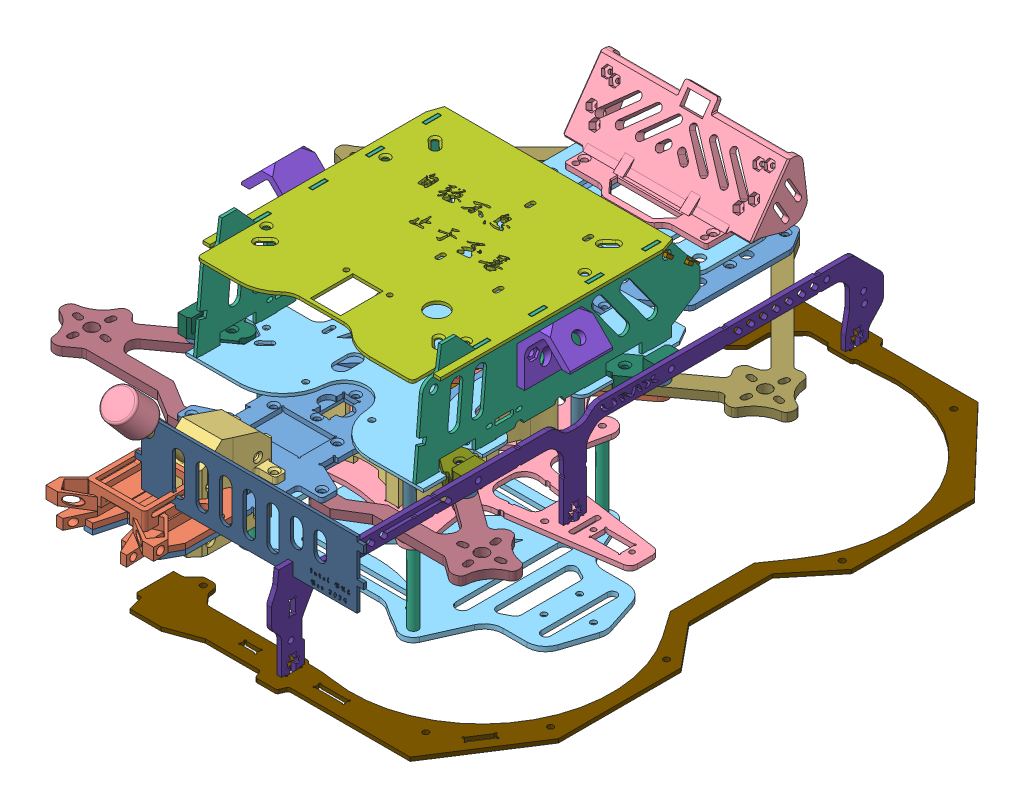
SolidWorks assembly 【Intel NUC】Chimera_5_XMU, configuration 默认. Lengths in mm.
Overall size (348.29 148.9 341.57).
201 component instances, 54 part files, 112 mates.
Components (placement in the parent):
- 主结构1-1: 主结构1 [默认] at (1.5044 -10.0257 329.067) size (150.98 2.73 325.31)
- 主结构2-1: 主结构2 [默认] at (1.5044 -14.5257 329.067) x (1 0 0) z (0 -1 0) size (150.98 112.29 2.5)
- [打印]飞塔保护壳-1: [打印]飞塔保护壳 [默认] at (1.5044 -17.0257 329.067) size (76.01 41.7 83)
- 底板_1-1: 底板_1 [默认] at (1.5044 -47.5257 329.067) size (209.17 2.5 135.35)
- 电池板SLDPRT-1: 电池板SLDPRT [默认] at (1.5044 -90.0257 329.067) size (187.98 2.5 112.92)
- 铝柱_40mm-5: 铝柱_40mm [默认] at (43.5044 -87.5257 279.067) x (0.657496 0 -0.753458) z (0 1 0) size (5 5 40)
- 铝柱_40mm-8: 铝柱_40mm [默认] at (-40.4956 -87.5257 279.067) x (-0.934177 0 -0.35681) z (0 1 0) size (5 5 40)
- 铝柱_40mm-9: 铝柱_40mm [默认] at (-40.4956 -87.5257 379.067) x (-0.934177 0 -0.35681) z (0 1 0) size (5 5 40)
- 铝柱_40mm-10: 铝柱_40mm [默认] at (43.5044 -87.5257 379.067) x (-0.903539 0 -0.428507) z (0 1 0) size (5 5 40)
- Air Unit.step-1: Air Unit.step [默认] at (8.357 -13.0257 442.2598) x (0 -1 0) z (0 0 -1) size (30.99 15 32.5) (hidden)
  - Bottom Case.step-1: Bottom Case.step [默认] at origin size (30.5 3.8 32.5)
  - Mid Case.step-1: Mid Case.step [默认] at origin size (30.5 12 32.5)
  - Top Case.step-1: Top Case.step [默认] at origin size (30.99 7.25 32.5)
  - Internal.step-1: Internal.step [默认] at origin size (29.25 12.4 30.75)
  - Screws.step-1: Screws.step [默认] at origin size (28.5 14.75 28.5)
- F45A.STEP-1: F45A.STEP [默认] at (2.5197 -30.0482 327.7528) size (44 7.18 42)
  - F45A PCB.STEP-1: F45A PCB.STEP [默认] at origin size (44 3.01 42)
  - DF13-10P.STEP-1: DF13-10P.STEP [默认] at (3.125 2.88 -16.6) x (-1 0 0) z (0 0 -1) size (14.25 3.58 5.1)
  - Heat Sink.STEP-1: Heat Sink.STEP [默认] at (0 2.5 0) size (37 3 37)
  - TPH1R403NL.STEP-1: TPH1R403NL.STEP [默认] at (8.2237 -1 16.1) x (0 0 -1) z (-1 0 0) size (5.3 1 6)
  - TPH1R403NL.STEP-2: TPH1R403NL.STEP [默认] at (8.5237 -1 9.95) x (-1 0 0) z (0 0 1) size (5.3 1 6)
  - TPH1R403NL.STEP-3: TPH1R403NL.STEP [默认] at (14.6737 -1 9.0737) x (0 0 1) z (1 0 0) size (5.3 1 6)
  - TPH1R403NL.STEP-4: TPH1R403NL.STEP [默认] at (14.6737 -1 2.8237) x (0 0 1) z (1 0 0) size (5.3 1 6)
  - TPH1R403NL.STEP-5: TPH1R403NL.STEP [默认] at (-8.2237 -1 16.1) x (0 0 1) z (1 0 0) size (5.3 1 6)
  - TPH1R403NL.STEP-6: TPH1R403NL.STEP [默认] at (-14.6737 -1 2.8237) x (0 0 -1) z (-1 0 0) size (5.3 1 6)
  - TPH1R403NL.STEP-7: TPH1R403NL.STEP [默认] at (-14.6737 -1 9.0737) x (0 0 -1) z (-1 0 0) size (5.3 1 6)
  - TPH1R403NL.STEP-8: TPH1R403NL.STEP [默认] at (8.2237 -1 -16.1) x (0 0 -1) z (-1 0 0) size (5.3 1 6)
  - TPH1R403NL.STEP-9: TPH1R403NL.STEP [默认] at (14.6737 -1 -2.8237) x (0 0 1) z (1 0 0) size (5.3 1 6)
  - TPH1R403NL.STEP-10: TPH1R403NL.STEP [默认] at (14.6737 -1 -9.0737) x (0 0 1) z (1 0 0) size (5.3 1 6)
  - TPH1R403NL.STEP-11: TPH1R403NL.STEP [默认] at (-8.2237 -1 -16.1) x (0 0 1) z (1 0 0) size (5.3 1 6)
  - TPH1R403NL.STEP-12: TPH1R403NL.STEP [默认] at (-14.6737 -1 -2.8237) x (0 0 -1) z (-1 0 0) size (5.3 1 6)
  - TPH1R403NL.STEP-13: TPH1R403NL.STEP [默认] at (-14.6737 -1 -9.0737) x (0 0 -1) z (-1 0 0) size (5.3 1 6)
  - TPH1R403NL.STEP-14: TPH1R403NL.STEP [默认] at (-8.5237 -1 9.95) x (-1 0 0) z (0 0 1) size (5.3 1 6)
  - TPH1R403NL.STEP-15: TPH1R403NL.STEP [默认] at (-8.5237 -1 -9.95) x (1 0 0) z (0 0 -1) size (5.3 1 6)
  - TPH1R403NL.STEP-16: TPH1R403NL.STEP [默认] at (8.5237 -1 -9.95) x (1 0 0) z (0 0 -1) size (5.3 1 6)
  - Capacitor.STEP-1: Capacitor.STEP [默认] at (9.5737 -1 -1.95) x (-1 0 0) z (0 0 1) size (3.2 1.5 1.6)
  - Capacitor.STEP-2: Capacitor.STEP [默认] at (9.5737 -1 -0.15) x (-1 0 0) z (0 0 1) size (3.2 1.5 1.6)
  - Capacitor.STEP-3: Capacitor.STEP [默认] at (9.5737 -1 1.65) x (-1 0 0) z (0 0 1) size (3.2 1.5 1.6)
  - Capacitor.STEP-4: Capacitor.STEP [默认] at (9.5737 -1 3.45) x (-1 0 0) z (0 0 1) size (3.2 1.5 1.6)
  - Capacitor.STEP-5: Capacitor.STEP [默认] at (-9.5737 -1 -1.95) x (-1 0 0) z (0 0 1) size (3.2 1.5 1.6)
  - Capacitor.STEP-6: Capacitor.STEP [默认] at (-9.5737 -1 -0.15) x (-1 0 0) z (0 0 1) size (3.2 1.5 1.6)
  - Capacitor.STEP-7: Capacitor.STEP [默认] at (-9.5737 -1 1.65) x (-1 0 0) z (0 0 1) size (3.2 1.5 1.6)
  - Capacitor.STEP-8: Capacitor.STEP [默认] at (-9.5737 -1 3.45) x (-1 0 0) z (0 0 1) size (3.2 1.5 1.6)
  - Capacitor.STEP-9: Capacitor.STEP [默认] at (5.3737 -1.8 -8.35) x (0 0 1) z (0 -1 0) size (3.2 1.5 1.6)
  - Capacitor.STEP-10: Capacitor.STEP [默认] at (3.5737 -1.8 -8.35) x (0 0 1) z (0 -1 0) size (3.2 1.5 1.6)
  - Capacitor.STEP-11: Capacitor.STEP [默认] at (1.7737 -1.8 -8.35) x (0 0 1) z (0 -1 0) size (3.2 1.5 1.6)
  - Capacitor.STEP-12: Capacitor.STEP [默认] at (-0.0263 -1.8 -8.35) x (0 0 1) z (0 -1 0) size (3.2 1.5 1.6)
  - Capacitor.STEP-13: Capacitor.STEP [默认] at (-1.8263 -1.8 -8.35) x (0 0 1) z (0 -1 0) size (3.2 1.5 1.6)
  - Capacitor.STEP-14: Capacitor.STEP [默认] at (5.3737 -1.8 10.75) x (0 0 1) z (0 -1 0) size (3.2 1.5 1.6)
  - Capacitor.STEP-15: Capacitor.STEP [默认] at (3.5737 -1.8 10.75) x (0 0 1) z (0 -1 0) size (3.2 1.5 1.6)
  - Capacitor.STEP-16: Capacitor.STEP [默认] at (1.7737 -1.8 10.75) x (0 0 1) z (0 -1 0) size (3.2 1.5 1.6)
  - Capacitor.STEP-17: Capacitor.STEP [默认] at (-0.0263 -1.8 10.75) x (0 0 1) z (0 -1 0) size (3.2 1.5 1.6)
  - Capacitor.STEP-18: Capacitor.STEP [默认] at (-1.8263 -1.8 10.75) x (0 0 1) z (0 -1 0) size (3.2 1.5 1.6)
  - Capacitor.STEP-19: Capacitor.STEP [默认] at (-4.4263 -2.5 10.75) x (0 0 1) z (-1 0 0) size (3.2 1.5 1.6)
- [云台板]思翼A8Mini-1: [云台板]思翼A8Mini [默认] at (1.5044 54.4743 329.0671) x (-1 0 -0.000003) z (0 -1 0) size (92.34 65.32 2) (hidden)
- 机臂2-1: 机臂2 [默认] at (1.5044 -10.0257 329.067) x (1 0 0) z (0 0 -1) size (93.94 4.5 157.55)
- 机臂2-3: 机臂2 [默认] at (1.5044 -14.5257 329.067) x (-1 0 0) z (0 0 -1) size (93.94 4.5 157.55)
- 机臂3-1: 机臂3 [默认] at (1.5044 -14.5257 329.067) size (93.8 4.5 97.35)
- 机臂3-2: 机臂3 [默认] at (1.5044 -10.0257 329.067) x (-1 0 0) z (0 0 1) size (93.8 4.5 97.35)
- 铝柱_35mm-1: 铝柱_35mm [默认] at (-30.4956 -10.0257 371.067) x (1 0 0) z (0 -1 0) size (5 5 35)
- 铝柱_35mm-2: 铝柱_35mm [默认] at (33.5044 -10.0257 371.067) x (1 0 0) z (0 -1 0) size (5 5 35)
- 铝柱_35mm-3: 铝柱_35mm [默认] at (-34.4956 -10.0257 286.067) x (1 0 0) z (0 -1 0) size (5 5 35)
- 铝柱_35mm-4: 铝柱_35mm [默认] at (37.5044 -10.0257 286.067) x (1 0 0) z (0 -1 0) size (5 5 35)
- [打印]防撞圈安装件-右前左后_安装调整-1: [打印]防撞圈安装件-右前左后_安装调整 [默认] at (61.729 -7.5257 285.3113) size (22.94 14.75 21.64) (hidden)
- [打印]防撞圈安装件-右前左后_安装调整-2: [打印]防撞圈安装件-右前左后_安装调整 [默认] at (-58.7202 -7.5257 372.8227) x (-1 0 0) z (0 0 -1) size (22.94 14.75 21.64)
- [打印]防撞圈安装件-左前右后_安装调整-1: [打印]防撞圈安装件-左前右后_安装调整 [默认] at (-58.7202 -7.5257 285.3113) size (22.94 14.75 21.64)
- [打印]防撞圈安装件-左前右后_安装调整-2: [打印]防撞圈安装件-左前右后_安装调整 [默认] at (61.729 -7.5257 372.8227) x (-1 0 0) z (0 0 -1) size (22.94 14.75 21.64) (hidden)
- 防撞圈固定板-1: 防撞圈固定板 [默认] at (76.5044 3.7243 329.067) x (0 0 -1) z (1 0 0) size (323.84 57.5 2.5)
- 防撞圈-2片式-1: 防撞圈-2片式 [默认] at (1.5044 -42.0257 329.067) x (0 0 -1) z (0 1 0) size (322.86 178.56 2)
- [pcb]分电PCB轮廓-1: [pcb]分电PCB轮廓 [默认] at (1.5044 -11.6257 337.2797) size (53.58 3 152.15)
- [打印]综合天线接口-5寸机_修改-1: [打印]综合天线接口-5寸机_修改 [默认] at (1.5044 -7.5257 329.067) size (57 20.5 61.52)
- [打印]o3支架-1: [打印]o3支架 [默认] at (1.5044 -13.0257 329.067) size (40.8 71.3 61.95)
- Antenna.step-1: Antenna.step [默认] at (1.5044 5.6745 451.7025) x (-0.985663 0.113991 -0.124399) z (0 -0.737277 -0.67559) size (17.31 17.31 63)
- 铝柱_30mm-1: 铝柱_30mm [默认] at (40.8394 -10.0257 208.8847) x (1 0 0) z (0 -1 0) size (5 5 30) (hidden)
- 铝柱_30mm-2: 铝柱_30mm [默认] at (16.1053 -10.0257 462.8732) x (-0.837169 0 -0.546944) z (0 -1 0) size (5 5 30) (hidden)
- [云台板]G-port云台结构-1: [云台板]G-port云台结构 [默认] at (1.5041 3.4743 329.0669) x (-1 0 -0.000003) z (0 -1 0) size (92.34 65.32 2)
- [打印]飞控转接板-1: [打印]飞控转接板 [默认] at (1.5044 -36.7457 329.067) x (1 0 0) z (0 -1 0) size (36.5 36.5 2)
- [云台板]astrorc单轴云台-2: [云台板]astrorc单轴云台 [默认] at (1.5044 0.9743 329.067) x (-1 0 0) z (0 -1 0) size (92.34 58.82 29.5) (hidden)
- MTF-01 Optical Flow &Lidar Sensor.step-1: MTF-01 Optical Flow &Lidar Sensor.step [默认] at (-13.1758 -52.2597 251.4922) x (0.999998 0 -0.002058) z (0 -1 0) size (29.45 17.1 14.23)
  - Board.step-1: Board.step [默认] at origin size (29.45 17.1 1.28)
    - Open CASCADE STEP translator 6.8 1.1.1.step-1: Open CASCADE STEP translator 6.8 1.1.1.step [默认] at (0 0 -1.279) size (29.45 17.1 1.28)
  - Open CASCADE STEP translator 6.8 1.2.step-1: Open CASCADE STEP translator 6.8 1.2.step [默认] at origin size (6 4.95 2.96)
    - SM04B-SRSS-TB.step-1: SM04B-SRSS-TB.step [默认] at (11.4779 13.1201 -0.979) x (1 0 0) z (0 1 0) size (6 2.96 4.95)
  - U5.step-1: U5.step [默认] at origin size (4.09 4.09 0.8)
    - QFN50P400X400X80-25N.step-1: QFN50P400X400X80-25N.step [默认] at (14.3501 5.7301 -1.279) x (0 -1 0) z (0 0 -1) size (4.09 4.09 0.8)
  - R17.step-1: R17.step [默认] at origin size (0.55 1.05 0.4)
    - RES_0402_(1005_metric).step-1: RES_0402_(1005_metric).step [默认] at (16.5751 15.6 -1.279) x (0 1 0) z (0 0 -1) size (1.05 0.55 0.4)
  - R16.step-1: R16.step [默认] at origin size (0.55 1.05 0.4)
    - RES_0402_(1005_metric).step-1: RES_0402_(1005_metric).step [默认] at (15.6251 15.6 -1.279) x (0 1 0) z (0 0 -1) size (1.05 0.55 0.4)
  - R15.step-1: R15.step [默认] at origin size (1.05 0.55 0.4)
    - RES_0402_(1005_metric).step-1: RES_0402_(1005_metric).step [默认] at (23.05 13.1499 0) x (-1 0 0) z (0 0 1) size (1.05 0.55 0.4)
  - R14.step-1: R14.step [默认] at origin size (1.05 0.55 0.4)
    - RES_0402_(1005_metric).step-1: RES_0402_(1005_metric).step [默认] at (14.45 11.0499 -1.279) x (1 0 0) z (0 0 -1) size (1.05 0.55 0.4)
  - R13.step-1: R13.step [默认] at origin size (1.05 0.55 0.4)
    - RES_0402_(1005_metric).step-1: RES_0402_(1005_metric).step [默认] at (21.75 6.7499 -1.279) x (1 0 0) z (0 0 -1) size (1.05 0.55 0.4)
  - R12.step-1: R12.step [默认] at origin size (1.05 0.55 0.4)
    - RES_0402_(1005_metric).step-1: RES_0402_(1005_metric).step [默认] at (12.75 0.8501 0) x (1 0 0) z (0 0 1) size (1.05 0.55 0.4)
  - R11.step-1: R11.step [默认] at origin size (1.05 0.55 0.4)
    - RES_0402_(1005_metric).step-1: RES_0402_(1005_metric).step [默认] at (11.95 0.9499 -1.279) x (1 0 0) z (0 0 -1) size (1.05 0.55 0.4)
  - R10.step-1: R10.step [默认] at origin size (0.55 1.05 0.4)
    - RES_0402_(1005_metric).step-1: RES_0402_(1005_metric).step [默认] at (18.1001 4.675 -1.279) x (0 1 0) z (0 0 -1) size (1.05 0.55 0.4)
  - R9.step-1: R9.step [默认] at origin size (0.55 1.05 0.4)
    - RES_0402_(1005_metric).step-1: RES_0402_(1005_metric).step [默认] at (11.3001 8.6 -1.279) x (0 1 0) z (0 0 -1) size (1.05 0.55 0.4)
  - R8.step-1: R8.step [默认] at origin size (0.55 1.05 0.4)
    - RES_0402_(1005_metric).step-1: RES_0402_(1005_metric).step [默认] at (18.4501 9.65 -1.279) x (0 1 0) z (0 0 -1) size (1.05 0.55 0.4)
  - R7.step-1: R7.step [默认] at origin size (0.55 1.05 0.4)
    - RES_0402_(1005_metric).step-1: RES_0402_(1005_metric).step [默认] at (17.3501 9.65 -1.279) x (0 1 0) z (0 0 -1) size (1.05 0.55 0.4)
  - R6.step-1: R6.step [默认] at origin size (0.55 1.05 0.4)
    - RES_0402_(1005_metric).step-1: RES_0402_(1005_metric).step [默认] at (16.3501 9.65 -1.279) x (0 1 0) z (0 0 -1) size (1.05 0.55 0.4)
  - R5.step-1: R5.step [默认] at origin size (0.55 1.05 0.4)
    - RES_0402_(1005_metric).step-1: RES_0402_(1005_metric).step [默认] at (15.3501 9.65 -1.279) x (0 1 0) z (0 0 -1) size (1.05 0.55 0.4)
  - R4.step-1: R4.step [默认] at origin size (0.55 1.05 0.4)
    - RES_0402_(1005_metric).step-1: RES_0402_(1005_metric).step [默认] at (14.3501 9.65 -1.279) x (0 1 0) z (0 0 -1) size (1.05 0.55 0.4)
  - R3.step-1: R3.step [默认] at origin size (0.55 1.05 0.4)
    - RES_0402_(1005_metric).step-1: RES_0402_(1005_metric).step [默认] at (13.3501 9.65 -1.279) x (0 1 0) z (0 0 -1) size (1.05 0.55 0.4)
  - R2.step-1: R2.step [默认] at origin size (0.55 1.05 0.4)
    - RES_0402_(1005_metric).step-1: RES_0402_(1005_metric).step [默认] at (12.3501 9.65 -1.279) x (0 1 0) z (0 0 -1) size (1.05 0.55 0.4)
  - R1.step-1: R1.step [默认] at origin size (1.05 0.55 0.4)
    - RES_0402_(1005_metric).step-1: RES_0402_(1005_metric).step [默认] at (21.75 15.0501 0) x (1 0 0) z (0 0 1) size (1.05 0.55 0.4)
  - D3.step-1: D3.step [默认] at origin size (5.7 5.3 12.2)
    - LED_5mm______.step-1: LED_5mm______.step [默认] at (19.65 5.55 0) x (0 1 0) z (0 0 1) size (5.3 5.7 8.7)
    - LED_5MM-W.step-1: LED_5MM-W.step [默认] at (19.65 5.55 0) x (0 1 0) z (0 0 1) size (4.06 1.6 7.95)
  - D2.step-1: D2.step [默认] at origin size (5.7 5.3 12.2)
    - LED_5MM-R.step-1: LED_5MM-R.step [默认] at (9.65 5.55 0) x (0 -1 0) z (0 0 1) size (4.06 1.6 7.95)
      - LED_5MM-R-5814_AF0_ASM.step-1: LED_5MM-R-5814_AF0_ASM.step [默认] at origin size (4.06 1.6 7.95)
        - LED_5MM-R-936_AF0.step-1: LED_5MM-R-936_AF0.step [默认] at origin size (4.06 1.6 7.95)
    - LED_5mm______.step-1: LED_5mm______.step [默认] at (9.65 5.55 0) x (0 -1 0) z (0 0 1) size (5.3 5.7 8.7)
  - D1.step-1: D1.step [默认] at origin size (1.6 0.8 0.75)
    - LED_0603_APT1608_BLUE.step-1: LED_0603_APT1608_BLUE.step [默认] at (21.7501 16.1501 0) x (1 0 0) z (0 0 1) size (1.6 0.8 0.75)
  - C28.step-1: C28.step [默认] at origin size (0.55 1.05 0.55)
    - CAP_0402_(1005_metric).step-1: CAP_0402_(1005_metric).step [默认] at (8.3501 11.65 0) x (0 -1 0) z (0 0 1) size (1.05 0.55 0.55)
  - C27.step-1: C27.step [默认] at origin size (1.05 0.55 0.55)
    - CAP_0402_(1005_metric).step-1: CAP_0402_(1005_metric).step [默认] at (15.45 12.0499 -1.279) x (1 0 0) z (0 0 -1) size (1.05 0.55 0.55)
  - C26.step-1: C26.step [默认] at origin size (1.05 0.55 0.55)
    - CAP_0402_(1005_metric).step-1: CAP_0402_(1005_metric).step [默认] at (15.45 12.9501 -1.279) x (-1 0 0) z (0 0 -1) size (1.05 0.55 0.55)
  - C25.step-1: C25.step [默认] at origin size (1.05 0.55 0.55)
    - CAP_0402_(1005_metric).step-1: CAP_0402_(1005_metric).step [默认] at (9.85 13.5501 0) x (1 0 0) z (0 0 1) size (1.05 0.55 0.55)
  - C24.step-1: C24.step [默认] at origin size (0.9 1.7 0.9)
    - CAP_0603.step-1: CAP_0603.step [默认] at (9.8499 11.55 -0.013) x (0 1 0) z (0 0 1) size (1.7 0.9 0.9)
  - C23.step-1: C23.step [默认] at origin size (0.55 1.05 0.55)
    - CAP_0402_(1005_metric).step-1: CAP_0402_(1005_metric).step [默认] at (10.4499 15.35 0) x (0 1 0) z (0 0 1) size (1.05 0.55 0.55)
  - C21.step-1: C21.step [默认] at origin size (0.9 1.7 0.9)
    - CAP_0603.step-1: CAP_0603.step [默认] at (9.2499 15.55 -0.013) x (0 1 0) z (0 0 1) size (1.7 0.9 0.9)
  - C20.step-1: C20.step [默认] at origin size (0.55 1.05 0.55)
    - CAP_0402_(1005_metric).step-1: CAP_0402_(1005_metric).step [默认] at (15.5501 1.75 0) x (0 -1 0) z (0 0 1) size (1.05 0.55 0.55)
  - C19.step-1: C19.step [默认] at origin size (1.05 0.55 0.55)
    - CAP_0402_(1005_metric).step-1: CAP_0402_(1005_metric).step [默认] at (14.35 2.3501 -1.279) x (-1 0 0) z (0 0 -1) size (1.05 0.55 0.55)
  - C18.step-1: C18.step [默认] at origin size (0.9 1.7 0.9)
    - CAP_0603.step-1: CAP_0603.step [默认] at (14.4501 1.55 -0.013) x (0 -1 0) z (0 0 1) size (1.7 0.9 0.9)
  - C17.step-1: C17.step [默认] at origin size (1.7 0.9 0.9)
    - CAP_0603.step-1: CAP_0603.step [默认] at (14.5 1.0501 -1.266) x (-1 0 0) z (0 0 -1) size (1.7 0.9 0.9)
  - C16.step-1: C16.step [默认] at origin size (0.55 1.05 0.55)
    - CAP_0402_(1005_metric).step-1: CAP_0402_(1005_metric).step [默认] at (19.7501 1.95 -1.279) x (0 1 0) z (0 0 -1) size (1.05 0.55 0.55)
  - C15.step-1: C15.step [默认] at origin size (1.45 2.2 1.35)
    - CAP_0805.step-1: CAP_0805.step [默认] at (16.9501 1.8501 -1.266) x (0 1 0) z (0 0 -1) size (2.2 1.45 1.35)
  - C14.step-1: C14.step [默认] at origin size (0.9 1.7 0.9)
    - CAP_0603.step-1: CAP_0603.step [默认] at (18.5501 1.75 -1.266) x (0 1 0) z (0 0 -1) size (1.7 0.9 0.9)
  - C13.step-1: C13.step [默认] at origin size (1.7 0.9 0.9)
    - CAP_0603.step-1: CAP_0603.step [默认] at (11.65 2.4499 -1.266) x (1 0 0) z (0 0 -1) size (1.7 0.9 0.9)
  - C12.step-1: C12.step [默认] at origin size (1.05 0.55 0.55)
    - CAP_0402_(1005_metric).step-1: CAP_0402_(1005_metric).step [默认] at (23.05 12.0501 0) x (1 0 0) z (0 0 1) size (1.05 0.55 0.55)
  - C11.step-1: C11.step [默认] at origin size (1.05 0.55 0.55)
    - CAP_0402_(1005_metric).step-1: CAP_0402_(1005_metric).step [默认] at (19.25 16.3499 0) x (-1 0 0) z (0 0 1) size (1.05 0.55 0.55)
  - C10.step-1: C10.step [默认] at origin size (1.05 0.55 0.55)
    - CAP_0402_(1005_metric).step-1: CAP_0402_(1005_metric).step [默认] at (20.75 10.5499 0) x (-1 0 0) z (0 0 1) size (1.05 0.55 0.55)
  - C8.step-1: C8.step [默认] at origin size (1.7 0.9 0.9)
    - CAP_0603.step-1: CAP_0603.step [默认] at (7.15 15.6501 -0.013) x (1 0 0) z (0 0 1) size (1.7 0.9 0.9)
  - C7.step-1: C7.step [默认] at origin size (1.7 0.9 0.9)
    - CAP_0603.step-1: CAP_0603.step [默认] at (23.15 5.2501 -1.266) x (-1 0 0) z (0 0 -1) size (1.7 0.9 0.9)
  - C6.step-1: C6.step [默认] at origin size (1.05 0.55 0.55)
    - CAP_0402_(1005_metric).step-1: CAP_0402_(1005_metric).step [默认] at (23.25 10.8501 -1.279) x (-1 0 0) z (0 0 -1) size (1.05 0.55 0.55)
  - C5.step-1: C5.step [默认] at origin size (0.9 1.7 0.9)
    - CAP_0603.step-1: CAP_0603.step [默认] at (20.1499 9.5 -1.266) x (0 -1 0) z (0 0 -1) size (1.7 0.9 0.9)
  - C4.step-1: C4.step [默认] at origin size (0.9 1.7 0.9)
    - CAP_0603.step-1: CAP_0603.step [默认] at (10.0501 10.35 -1.266) x (0 1 0) z (0 0 -1) size (1.7 0.9 0.9)
  - C3.step-1: C3.step [默认] at origin size (0.55 1.05 0.55)
    - CAP_0402_(1005_metric).step-1: CAP_0402_(1005_metric).step [默认] at (8.6501 11.85 -1.279) x (0 1 0) z (0 0 -1) size (1.05 0.55 0.55)
  - C2.step-1: C2.step [默认] at origin size (0.55 1.05 0.55)
    - CAP_0402_(1005_metric).step-1: CAP_0402_(1005_metric).step [默认] at (7.1501 13.15 -1.279) x (0 1 0) z (0 0 -1) size (1.05 0.55 0.55)
  - C1.step-1: C1.step [默认] at origin size (0.9 1.7 0.9)
    - CAP_0603.step-1: CAP_0603.step [默认] at (5.9501 13.5 -1.266) x (0 1 0) z (0 0 -1) size (1.7 0.9 0.9)
  - Free-Models.step-1: Free-Models.step [默认] at origin size (18.05 14.8 10)
    - lens_chip_package.step-1: lens_chip_package.step [默认] at (14.7574 16.3068 -0.127) x (0 -1 0) z (-1 0 0) size (6 5.08 6)
      - LENS.step-1: LENS.step [默认] at origin size (3.8 3.95 3.8)
        - Open CASCADE STEP translator 6.8 1.50.3.1.1.step-1: Open CASCADE STEP translator 6.8 1.50.3.1.1.step [默认] at origin size (3.8 1.95 3.8)
        - Open CASCADE STEP translator 6.8 1.50.3.1.2.step-1: Open CASCADE STEP translator 6.8 1.50.3.1.2.step [默认] at origin size (2.37 3.08 2.37)
      - NONE.step-1: NONE.step [默认] at origin size (6 2.28 6)
    - ____&______.step-1: ____&______.step [默认] at (19.6718 5.5748 0) x (-1 0 0) z (0 0 -1) size (8 8 10)
    - ____&______.step-2: ____&______.step [默认] at (9.6266 5.524 0) x (-1 0 0) z (0 0 -1) size (8 8 10)
- 铝柱_40mm-11: 铝柱_40mm [默认] at (-85.7956 -47.5257 329.067) x (1 0 0) z (0 -1 0) size (5 5 40)
- [打印]G-port云台板双目接驳件-1: [打印]G-port云台板双目接驳件 [默认] at (1.5041 3.4743 329.0669) x (1 0 0.000003) z (0 1 0) size (100 46.6 38.07)
- [打印]防撞圈安装件-右前左后_安装调整-3: [打印]防撞圈安装件-右前左后_安装调整 [默认] at (61.729 -7.5307 285.3113) size (22.94 14.75 21.64)
- [打印]防撞圈安装件-左前右后_安装调整-3: [打印]防撞圈安装件-左前右后_安装调整 [默认] at (61.88 -7.5257 372.8227) x (-1 0 0) z (0 0 -1) size (22.94 14.75 21.64)
- Shell_Bottom_NUC-1: Shell_Bottom_NUC [Default] at (1.5044 -7.5257 339.5893) x (1 0 0) z (0 0 1) size (125.5 1.6 155.37)
- Shell_Side_X2_NUC-1: Shell_Side_X2_NUC [默认] at (-57.3456 -5.9257 297.9276) x (1 0 0) z (0 0 1) size (1.6 59.1 150.28)
- Shell_Side_X2_NUC-2: Shell_Side_X2_NUC [默认] at (58.7544 -5.9257 297.9276) x (1 0 0) z (0 0 1) size (1.6 59.1 150.28)
- Shell_Top_NUC-1: Shell_Top_NUC [默认] at (1.5044 39.0743 322.9093) x (1 0 0) z (0 0 1) size (125.7 1.6 134.36)
- 天线基座-3D打印-通用-1: 天线基座-3D打印-通用 [默认] at (-71.5986 31.9757 318.5893) x (1 0 0) z (0 0 1) size (28.11 34.12 22.5)
- 天线基座-3D打印-通用-2: 天线基座-3D打印-通用 [默认] at (74.6075 31.9757 341.0893) x (-1 0 0) z (0 0 -1) size (28.11 34.12 22.5)
- 前盖_NUC-1: 前盖_NUC [默认] at (1.5044 32.4779 259.7695) x (1 0 0) z (0 -0.789337 0.61396) size (150.46 28.3 1.6)
- 后盖_NUC-1: 后盖_NUC [默认] at (55.9794 32.1768 476.7376) size (158 35.1 1.6)
Mates (geometry in assembly coordinates):
- 同心75: concentric anti-aligned: cylinder of 主结构1-1 through (16.7544 -7.5257 313.817) axis (0 -1 0) radius 1.55; cylinder of 主结构2-1 through (16.7544 -17.0257 313.817) axis (0 1 0) radius 1.55
- 同心76: concentric anti-aligned: cylinder of 主结构1-1 through (-58.7202 -7.5257 372.8227) axis (0 -1 0) radius 1.55; cylinder of 机臂3-2 through (-58.7202 -14.5257 372.8227) axis (0 1 0) radius 1.55
- 重合80: coincident anti-aligned: plane of 主结构1-1 through (1.5044 -10.0257 113.8082) normal (0 -1 0); plane of 机臂3-2 through (-36.8355 -10.0257 356.9226) normal (0 1 0)
- 同心77: concentric anti-aligned: cylinder of 主结构1-1 through (61.729 -7.5257 285.3113) axis (0 -1 0) radius 1.55; cylinder of 机臂2-1 through (61.729 -14.5257 285.3113) axis (0 1 0) radius 1.55
- 同心78: concentric aligned: cylinder of 主结构1-1 through (45.5486 -7.5257 361.067) axis (0 -1 0) radius 1.55; cylinder of 机臂3-1 through (45.5486 -10.0257 361.067) axis (0 -1 0) radius 1.55
- 重合81: coincident anti-aligned: plane of 主结构2-1 through (1.5044 -14.5257 177.7429) normal (0 1 0); plane of 机臂3-1 through (39.8443 -14.5257 356.9226) normal (0 -1 0)
- 同心79: concentric anti-aligned: cylinder of 主结构2-1 through (-58.7202 -17.0257 372.8227) axis (0 1 0) radius 1.55; circle of 机臂3-2
- 重合83: coincident anti-aligned: plane of 主结构2-1 through (1.5044 -14.5257 177.7429) normal (0 1 0); plane of 机臂3-2 through (-36.8355 -14.5257 356.9226) normal (0 -1 0)
- 重合84: coincident anti-aligned: plane of 主结构2-1 through (1.5044 -14.5257 177.7429) normal (0 1 0); plane of 机臂2-3 through (1.5044 -14.5257 329.067) normal (0 -1 0)
- 同心80: concentric anti-aligned: cylinder of 主结构2-1 through (-58.7202 -17.0257 285.3113) axis (0 1 0) radius 1.55; cylinder of 机臂2-3 through (-58.7202 -10.0257 285.3113) axis (0 -1 0) radius 1.55
- 同心81: concentric anti-aligned: cylinder of 主结构2-1 through (-42.5398 -17.0257 297.067) axis (0 1 0) radius 1.55; cylinder of 机臂2-3 through (-42.5398 -10.0257 297.067) axis (0 -1 0) radius 1.55
- 同心82: concentric anti-aligned: cylinder of 主结构2-1 through (45.5486 -17.0257 361.067) axis (0 1 0) radius 1.55; cylinder of 机臂3-1 through (45.5486 -10.0257 361.067) axis (0 -1 0) radius 1.55
- 同心83: concentric anti-aligned: cylinder of 主结构2-1 through (61.729 -17.0257 372.8227) axis (0 1 0) radius 1.55; cylinder of 机臂3-1 through (61.729 -10.0257 372.8227) axis (0 -1 0) radius 1.55
- 重合85: coincident anti-aligned: plane of 主结构2-1 through (1.5044 -14.5257 177.7429) normal (0 1 0); plane of 机臂3-1 through (39.8443 -14.5257 356.9226) normal (0 -1 0)
- 同心84: concentric aligned: cylinder of 主结构1-1 through (45.5486 -7.5257 361.067) axis (0 -1 0) radius 1.55; cylinder of 机臂3-1 through (45.5486 -10.0257 361.067) axis (0 -1 0) radius 1.55
- 同心85: concentric aligned: cylinder of 主结构1-1 through (61.729 -7.5257 372.8227) axis (0 -1 0) radius 1.55; cylinder of 机臂3-1 through (61.729 -10.0257 372.8227) axis (0 -1 0) radius 1.55
- 重合86: coincident anti-aligned: plane of 主结构1-1 through (1.5044 -10.0257 113.8082) normal (0 -1 0); plane of 机臂3-1 through (39.8443 -10.0257 356.9226) normal (0 1 0)
- 同心86: concentric anti-aligned: cylinder of 主结构1-1 through (37.5044 -7.5257 286.067) axis (0 -1 0) radius 1.55; cylinder of 铝柱_35mm-4 through (37.5044 -45.0257 286.067) axis (0 1 0) radius 1.55
- 重合87: coincident anti-aligned: plane of 主结构1-1 through (1.5044 -10.0257 113.8082) normal (0 -1 0); plane of 铝柱_35mm-4 through (37.5044 -10.0257 286.067) normal (0 1 0)
- 同心87: concentric anti-aligned: cylinder of 主结构1-1 through (-34.4956 -7.5257 286.067) axis (0 -1 0) radius 1.55; cylinder of 铝柱_35mm-3 through (-34.4956 -45.0257 286.067) axis (0 1 0) radius 1.55
- 重合88: coincident anti-aligned: plane of 主结构1-1 through (1.5044 -10.0257 113.8082) normal (0 -1 0); plane of 铝柱_35mm-3 through (-34.4956 -10.0257 286.067) normal (0 1 0)
- 同心88: concentric anti-aligned: cylinder of 主结构1-1 through (-30.4956 -7.5257 371.067) axis (0 -1 0) radius 1.55; cylinder of 铝柱_35mm-1 through (-30.4956 -45.0257 371.067) axis (0 1 0) radius 1.55
- 重合89: coincident anti-aligned: plane of 主结构1-1 through (1.5044 -10.0257 113.8082) normal (0 -1 0); plane of 铝柱_35mm-1 through (-30.4956 -10.0257 371.067) normal (0 1 0)
- 同心89: concentric anti-aligned: cylinder of 主结构1-1 through (33.5044 -7.5257 371.067) axis (0 -1 0) radius 1.55; cylinder of 铝柱_35mm-2 through (33.5044 -45.0257 371.067) axis (0 1 0) radius 1.55
- 重合90: coincident anti-aligned: plane of 主结构1-1 through (1.5044 -10.0257 113.8082) normal (0 -1 0); plane of 铝柱_35mm-2 through (33.5044 -10.0257 371.067) normal (0 1 0)
- 同心90: concentric anti-aligned: cylinder of 底板_1-1 through (33.5044 -45.0257 371.067) axis (0 -1 0) radius 1.55; cylinder of 铝柱_35mm-2 through (33.5044 -45.0257 371.067) axis (0 1 0) radius 1.55
- 同心91: concentric anti-aligned: cylinder of 底板_1-1 through (-30.4956 -45.0257 371.067) axis (0 -1 0) radius 1.55; cylinder of 铝柱_35mm-1 through (-30.4956 -45.0257 371.067) axis (0 1 0) radius 1.55
- 重合91: coincident anti-aligned: plane of 底板_1-1 through (-244.6747 -45.0257 329.067) normal (0 1 0); plane of 铝柱_35mm-1 through (-30.4956 -45.0257 371.067) normal (0 -1 0)
- 距离1: distance = 3.75 mm anti-aligned: plane of Air Unit.step-1/Top Case.step-1 through (-6.143 -13.0257 442.2598) normal (-1 0 0); plane of 主结构1-1 through (-9.893 -7.5257 456.5808) normal (1 0 0)
- 重合95: coincident anti-aligned: plane of 底板_1-1 through (-244.6747 -47.5257 329.067) normal (0 -1 0); plane of 铝柱_40mm-9 through (-40.4956 -47.5257 379.067) normal (0 1 0)
- 重合96: coincident anti-aligned: plane of 底板_1-1 through (-244.6747 -47.5257 329.067) normal (0 -1 0); plane of 铝柱_40mm-10 through (43.5044 -47.5257 379.067) normal (0 1 0)
- 重合97: coincident anti-aligned: plane of 底板_1-1 through (-244.6747 -47.5257 329.067) normal (0 -1 0); plane of 铝柱_40mm-5 through (43.5044 -47.5257 279.067) normal (0 1 0)
- 重合99: coincident anti-aligned: plane of 底板_1-1 through (-244.6747 -47.5257 329.067) normal (0 -1 0); plane of 铝柱_40mm-8 through (-40.4956 -47.5257 279.067) normal (0 1 0)
- 重合100: coincident anti-aligned: plane of 电池板SLDPRT-1 through (1.5044 -87.5257 217.5353) normal (0 1 0); plane of 铝柱_40mm-8 through (-40.4956 -87.5257 279.067) normal (0 -1 0)
- 重合101: coincident anti-aligned: plane of 主结构1-1 through (1.5044 -7.5257 113.8082) normal (0 1 0); plane of [打印]防撞圈安装件-1 through (58.6606 -7.5257 287.5406) normal (0 -1 0)
- 同心93: concentric aligned: cylinder of 主结构1-1 through (61.729 -7.5257 285.3113) axis (0 -1 0) radius 1.55; cylinder of [打印]防撞圈安装件-1 through (61.729 -5.0257 285.3113) axis (0 -1 0) radius 1.55
- 同心96: concentric aligned: cylinder of 主结构1-1 through (-58.7202 -7.5257 372.8227) axis (0 -1 0) radius 1.55; cylinder of [打印]防撞圈安装件-右前左后-2 through (-58.7202 -5.0257 372.8227) axis (0 -1 0) radius 1.55
- 平行6: parallel aligned: plane of 主结构1-1 through (-56.2656 -7.5257 376.9106) normal (0.587785 0 0.809017); plane of [打印]防撞圈安装件-右前左后-2 through (-51.3904 -12.5257 376.4588) normal (0.587785 0 0.809017)
- 同心97: concentric aligned: cylinder of 主结构1-1 through (-58.7202 -7.5257 285.3113) axis (0 -1 0) radius 1.55; cylinder of [打印]防撞圈安装件-左前右后-1 through (-58.7202 -5.0257 285.3113) axis (0 -1 0) radius 1.55
- 平行7: parallel aligned: plane of 主结构1-1 through (-72.0294 -7.5257 281.5129) normal (-0.587785 0 0.809017); plane of [打印]防撞圈安装件-左前右后-1 through (-59.9132 -12.5257 293.4059) normal (-0.587785 0 0.809017)
- 重合103: coincident anti-aligned: plane of 主结构1-1 through (1.5044 -7.5257 113.8082) normal (0 1 0); plane of [打印]防撞圈安装件-左前右后-1 through (-55.6518 -7.5257 287.5406) normal (0 -1 0)
- 同心98: concentric aligned: cylinder of 主结构1-1 through (61.729 -7.5257 372.8227) axis (0 -1 0) radius 1.55; cylinder of [打印]防撞圈安装件-左前右后-2 through (61.729 -5.0257 372.8227) axis (0 -1 0) radius 1.55
- 平行8: parallel aligned: plane of 主结构1-1 through (59.2744 -7.5257 376.9106) normal (-0.587785 0 0.809017); plane of [打印]防撞圈安装件-左前右后-2 through (54.3992 -12.5257 376.4588) normal (-0.587785 0 0.809017)
- 重合105: coincident anti-aligned: plane of [打印]防撞圈安装件-左前右后-2 through (58.6606 -7.5257 370.5934) normal (0 -1 0); plane of 主结构1-1 through (1.5044 -7.5257 113.8082) normal (0 1 0)
- 距离2: distance = 0.15 mm anti-aligned: plane of 防撞圈固定板-1 through (79.0044 3.7243 329.067) normal (1 0 0); plane of 底板_1-1 through (79.1544 -45.0257 331.2188) normal (-1 0 0)
- 距离3: distance = 0.5 mm anti-aligned: plane of 防撞圈固定板-1 through (79.0044 -45.0257 325.567) normal (0 0 -1); plane of 底板_1-1 through (76.3544 -45.0257 325.067) normal (0 0 1)
- 重合108: coincident aligned: plane of 底板_1-1 through (-244.6747 -47.5257 329.067) normal (0 -1 0); plane of 防撞圈固定板-1 through (79.0044 -47.5257 327.517) normal (0 -1 0)
- 重合115: coincident anti-aligned: plane of 防撞圈固定板-1 through (79.0044 -40.0257 474.817) normal (0 -1 0); plane of 防撞圈-2片式-1 through (104.733 -40.0257 404.067) normal (0 1 0)
- 距离6: distance = 0.5 mm anti-aligned: plane of 防撞圈固定板-1 through (76.5044 3.7243 329.067) normal (-1 0 0); plane of 防撞圈-2片式-1 through (76.0044 -40.0257 183.817) normal (1 0 0)
- 距离5: distance = 0.5 mm anti-aligned: plane of 防撞圈固定板-1 through (79.0044 -40.0257 176.317) normal (0 0 -1); plane of 防撞圈-2片式-1 through (76.0044 -40.0257 175.817) normal (0 0 1)
- 同心99: concentric aligned: cylinder of 主结构1-1 through (1.5044 -7.5257 388.067) axis (0 -1 0) radius 1.55; cylinder of [pcb]分电PCB轮廓-1 through (1.5044 -10.0257 388.067) axis (0 -1 0) radius 1.55
- 同心100: concentric aligned: cylinder of 主结构1-1 through (1.5044 -7.5257 367.567) axis (0 -1 0) radius 1.55; cylinder of [pcb]分电PCB轮廓-1 through (1.5044 -10.0257 367.567) axis (0 -1 0) radius 1.55
- 重合116: coincident anti-aligned: plane of 主结构1-1 through (1.5044 -7.5257 113.8082) normal (0 1 0); plane of [打印]综合天线接口-5寸机-1 through (-6.518 -7.5257 452.8141) normal (0 -1 0)
- 同心101: concentric aligned: cylinder of 主结构1-1 through (-20.8855 -7.5257 462.8732) axis (0 -1 0) radius 1.55; cylinder of [打印]综合天线接口-5寸机-1 through (-20.8855 -4.5257 462.8732) axis (0 -1 0) radius 1.55
- 距离7: distance = 1 mm anti-aligned: plane of [打印]o3支架-1 through (1.5044 -31.2757 421.7598) normal (0 0 -1); plane of 主结构1-1 through (-7.9956 -7.5257 420.7598) normal (0 0 1)
- 距离8: distance = 0.5 mm anti-aligned: plane of 主结构1-1 through (12.8999 -7.5257 452.7032) normal (-0.999459 0 0.032881); plane of [打印]o3支架-1 through (8.3248 -31.2757 328.8426) normal (0.999459 0 -0.032881)
- 平行10: parallel anti-aligned: plane of 主结构1-1 through (-9.8911 -7.5257 452.7032) normal (0.999459 0 0.032881); plane of [打印]o3支架-1 through (-5.3159 -31.2757 328.8426) normal (-0.999459 0 -0.032881)
- 平行11: parallel anti-aligned: plane of [打印]o3支架-1 through (1.5044 36.9862 480.3945) normal (0 0.737277 0.67559); plane of Antenna.step-1 through (0.223 5.8227 451.5408) normal (0 -0.737277 -0.67559)
- 同心104: concentric anti-aligned: circle of Antenna.step-1; circle of [打印]o3支架-1
- 同心106: concentric aligned: circle of Air Unit.step-1/Screws.step-1; circle of [打印]o3支架-1
- 同心107: concentric anti-aligned: circle of Air Unit.step-1/Screws.step-1; circle of [打印]o3支架-1
- 重合125: coincident anti-aligned: plane of [打印]o3支架-1 through (1.5044 36.9862 480.3945) normal (0 0.737277 0.67559); circle of Antenna.step-1
- 重合126: coincident anti-aligned: plane of 主结构1-1 through (1.5044 -7.5257 113.8082) normal (0 1 0); plane of [打印]o3支架-1 through (1.5044 -7.5257 329.067) normal (0 -1 0)
- 重合127: coincident anti-aligned: plane of 主结构1-1 through (1.5044 -10.0257 113.8082) normal (0 -1 0); plane of 铝柱_30mm-2 through (16.1053 -10.0257 462.8732) normal (0 1 0)
- 同心108: concentric anti-aligned: cylinder of 主结构1-1 through (16.1053 -7.5257 462.8732) axis (0 -1 0) radius 1.55; cylinder of 铝柱_30mm-2 through (16.1053 -40.0257 462.8732) axis (0 1 0) radius 1.55
- 同心109: concentric anti-aligned: cylinder of 主结构1-1 through (40.8394 -7.5257 208.8847) axis (0 -1 0) radius 1.55; cylinder of 铝柱_30mm-1 through (40.8394 -40.0257 208.8847) axis (0 1 0) radius 1.55
- 重合128: coincident anti-aligned: plane of 主结构1-1 through (1.5044 -10.0257 113.8082) normal (0 -1 0); plane of 铝柱_30mm-1 through (40.8394 -10.0257 208.8847) normal (0 1 0)
- 距离10: distance = 60 mm anti-aligned: plane of 主结构1-1 through (1.5044 -7.5257 113.8082) normal (0 1 0); plane of [云台板]思翼A8Mini-1 through (-43.145 52.4743 231.4462) normal (0 -1 0)
- 同心110: concentric anti-aligned: circle of 主结构1-1; circle of [云台板]思翼A8Mini-1
- 同心111: concentric anti-aligned: circle of 主结构1-1; circle of [云台板]思翼A8Mini-1
- 同心113: concentric aligned: circle of [云台板]思翼A8Mini-1; circle of [云台板]G-port云台结构-1
- 同心114: concentric aligned: circle of [云台板]思翼A8Mini-1; circle of [云台板]G-port云台结构-1
- 平行15: parallel anti-aligned: plane of 主结构2-1 through (1.5044 -17.0257 177.7429) normal (0 -1 0); plane of 飞控转接板-1 through (-13.7456 -36.7457 344.317) normal (0 1 0)
- 同心116: concentric aligned: circle of 主结构2-1; circle of 飞控转接板-1
- 同心117: concentric aligned: circle of 主结构2-1; circle of 飞控转接板-1
- 平行17: parallel aligned: plane of 主结构1-1 through (1.5044 -7.5257 113.8082) normal (0 1 0); plane of [云台板]astrorc单轴云台-2 through (-120.6097 0.9743 212.9405) normal (0 1 0)
- 同心120: concentric anti-aligned: circle of 主结构1-1; circle of [云台板]astrorc单轴云台-2
- 同心121: concentric anti-aligned: circle of 主结构1-1; circle of [云台板]astrorc单轴云台-2
- 同心122: concentric anti-aligned: circle of 底板_1-1; circle of 电池板SLDPRT-1
- 同心123: concentric aligned: circle of 底板_1-1; circle of 电池板SLDPRT-1
- 同心139: concentric anti-aligned: cylinder of 底板_1-1 through (-85.7956 -45.0257 329.067) axis (0 -1 0) radius 1.55; cylinder of 铝柱_40mm-11 through (-85.7956 -87.5257 329.067) axis (0 1 0) radius 1.55
- 重合133: coincident anti-aligned: plane of 电池板SLDPRT-1 through (1.5044 -87.5257 217.5353) normal (0 1 0); plane of 铝柱_40mm-11 through (-85.7956 -87.5257 329.067) normal (0 -1 0)
- 距离14: distance = 6.5 mm anti-aligned: plane of [云台板]astrorc单轴云台-2 through (-120.6097 -1.0257 212.9405) normal (0 -1 0); plane of 主结构1-1 through (1.5044 -7.5257 113.8082) normal (0 1 0)
- 距离17: distance = 9 mm anti-aligned: plane of 主结构1-1 through (1.5044 -7.5257 113.8082) normal (0 1 0); plane of [云台板]G-port云台结构-1 through (-39.3801 1.4743 227.9) normal (0 -1 0)
- 同心150: concentric anti-aligned: cylinder of [云台板]G-port云台结构-1 through (-32.5455 1.4743 212.4845) axis (0 1 0) radius 1.55; cylinder of [打印]G-port云台板双目接驳件-1 through (-32.5455 6.2243 212.4845) axis (0 -1 0) radius 1.55
- 重合140: coincident anti-aligned: plane of [云台板]G-port云台结构-1 through (-39.3801 3.4743 227.9) normal (0 1 0); plane of [打印]G-port云台板双目接驳件-1 through (1.5041 3.4743 329.0669) normal (0 -1 0)
- 同心151: concentric anti-aligned: cylinder of [云台板]G-port云台结构-1 through (35.5545 1.4743 212.4847) axis (0 1 0) radius 1.55; cylinder of [打印]G-port云台板双目接驳件-1 through (35.5545 6.2243 212.4847) axis (0 -1 0) radius 1.55
- 重合144: coincident anti-aligned: cylinder of 防撞圈固定板-1 through (79.0044 -1.7757 380.1785) axis (-1 0 0) radius 1.55; circle of [打印]防撞圈安装件-左前右后_安装调整-3
- 同心159: concentric anti-aligned: cylinder of 底板_1-1 through (13.6544 44.3658 253.987) axis (0 -1 0) radius 1.925; cylinder of MTF-01 Optical Flow &Lidar Sensor.step-1/Board.step-1/Open CASCADE STEP translator 6.8 1.1.1.step-1 through (13.6544 -50.9807 253.987) axis (0 1 0) radius 1.25
- 距离18: distance = 0.5 mm: line of MTF-01 Optical Flow &Lidar Sensor.step-1/Open CASCADE STEP translator 6.8 1.2.step-1/SM04B-SRSS-TB.step-1 through (0.8284 -48.0257 264.2284) axis (-0.999998 0 0.002058); plane of 底板_1-1 through (-244.6747 -47.5257 329.067) normal (0 -1 0)
- 重合145: coincident anti-aligned: plane of 主结构1-1 through (1.5044 -7.5257 113.8082) normal (0 1 0); plane of [打印]防撞圈安装件-右前左后_安装调整-2 through (-55.6518 -7.5257 370.5934) normal (0 -1 0)
- 同心160: concentric aligned: cylinder of 主结构1-1 through (61.729 -7.5257 285.3113) axis (0 -1 0) radius 1.55; cylinder of [打印]防撞圈安装件-右前左后_安装调整-3 through (61.729 -5.0307 285.3113) axis (0 -1 0) radius 1.55
- 同心161: concentric anti-aligned: cylinder of 主结构1-1 through (-13.4956 -17.5257 275.567) axis (0 1 0) radius 1.55; cylinder of Shell_Bottom_NUC-1 through (-13.4956 -5.9257 275.567) axis (0 -1 0) radius 1.55
- 重合146: coincident anti-aligned: plane of 主结构1-1 through (1.5044 -7.5257 113.8082) normal (0 1 0); plane of Shell_Bottom_NUC-1 through (1.5044 -7.5257 339.5893) normal (0 -1 0)
- 同心162: concentric aligned: cylinder of 主结构1-1 through (-15.9956 -7.5257 376.567) axis (0 -1 0) radius 1.55; cylinder of Shell_Bottom_NUC-1 through (-15.9956 -5.9257 376.567) axis (0 -1 0) radius 1.55
- Coincident1: coincident anti-aligned: plane of Shell_Bottom_NUC-1 through (1.5044 -5.9257 339.5893) normal (0 1 0); plane of Shell_Side_X2_NUC-1 through (-55.7456 -5.9257 297.9276) normal (0 -1 0)
- Distance1: distance = 0.25 mm anti-aligned: plane of Shell_Side_X2_NUC-1 through (-57.3456 -5.9257 297.9276) normal (-1 0 0); plane of Shell_Bottom_NUC-1 through (-57.5956 -5.9257 339.5893) normal (1 0 0)
- Distance2: distance = 0.25 mm anti-aligned: plane of Shell_Bottom_NUC-1 through (1.5044 -5.9257 262.0893) normal (0 0 1); plane of Shell_Side_X2_NUC-1 through (-23.3193 -5.9257 262.3393) normal (0 0 -1)
- Coincident4: coincident anti-aligned: plane of Shell_Bottom_NUC-1 through (1.5044 -5.9257 339.5893) normal (0 1 0); plane of Shell_Side_X2_NUC-2 through (60.3544 -5.9257 297.9276) normal (0 -1 0)
- Distance3: distance = 0.25 mm anti-aligned: plane of Shell_Side_X2_NUC-2 through (92.7807 -5.9257 270.3393) normal (0 0 1); plane of Shell_Bottom_NUC-1 through (1.5044 -5.9257 270.5893) normal (0 0 -1)
- Distance4: distance = 0.25 mm: plane of Shell_Side_X2_NUC-2 through (60.3544 -5.9257 297.9276) normal (1 0 0); line of Shell_Bottom_NUC-1 through (60.6044 -7.5257 262.0893) axis (0 0 1)
- Coincident5: coincident anti-aligned: plane of Shell_Side_X2_NUC-1 through (-55.7456 39.0743 297.9276) normal (0 1 0); plane of Shell_Top_NUC-1 through (1.5044 39.0743 322.9093) normal (0 -1 0)
- Distance5: distance = 0.25 mm anti-aligned: plane of Shell_Top_NUC-1 through (-55.4956 40.6743 383.5343) normal (-1 0 0); plane of Shell_Side_X2_NUC-1 through (-55.7456 -5.9257 297.9276) normal (1 0 0)
- Distance6: distance = 0.25 mm anti-aligned: plane of Shell_Top_NUC-1 through (-57.5956 40.6743 354.9843) normal (0 0 1); plane of Shell_Side_X2_NUC-1 through (-23.3193 -5.9257 355.2343) normal (0 0 -1)
- Coincident8: coincident anti-aligned: plane of Shell_Side_X2_NUC-2 through (60.3544 -5.9257 297.9276) normal (1 0 0); plane of 天线基座-3D打印-通用-2 through (60.3544 31.9757 318.5893) normal (-1 0 0)
- Concentric1: concentric anti-aligned: cylinder of Shell_Side_X2_NUC-2 through (58.7544 26.7257 323.3393) axis (1 0 0) radius 1.575; circle of 天线基座-3D打印-通用-2
- Coincident9: coincident anti-aligned: cylinder of Shell_Side_X2_NUC-2 through (58.7544 26.7257 336.3393) axis (1 0 0) radius 1.575; circle of 天线基座-3D打印-通用-2
- Coincident10: coincident anti-aligned: plane of Shell_Side_X2_NUC-1 through (-57.3456 -5.9257 297.9276) normal (-1 0 0); plane of 天线基座-3D打印-通用-1 through (-57.3456 31.9757 341.0893) normal (1 0 0)
- Coincident11: coincident aligned: cylinder of Shell_Side_X2_NUC-1 through (-57.3456 26.7257 323.3393) axis (1 0 0) radius 1.575; circle of 天线基座-3D打印-通用-1
- Concentric2: concentric aligned: cylinder of Shell_Side_X2_NUC-1 through (-57.3456 26.7257 336.3393) axis (1 0 0) radius 1.575; cylinder of 天线基座-3D打印-通用-1 through (-85.4579 26.7257 336.3393) axis (1 0 0) radius 1.575
- Concentric3: concentric aligned: circle of Shell_Side_X2_NUC-2; line of 前盖_NUC-1 through (62.0044 33.0743 261.8393) axis (1 0 0)
- Coincident12: coincident aligned: plane of Shell_Top_NUC-1 through (58.5044 40.6743 273.4843) normal (1 0 0); plane of 前盖_NUC-1 through (58.5044 31.2149 260.7518) normal (1 0 0)
